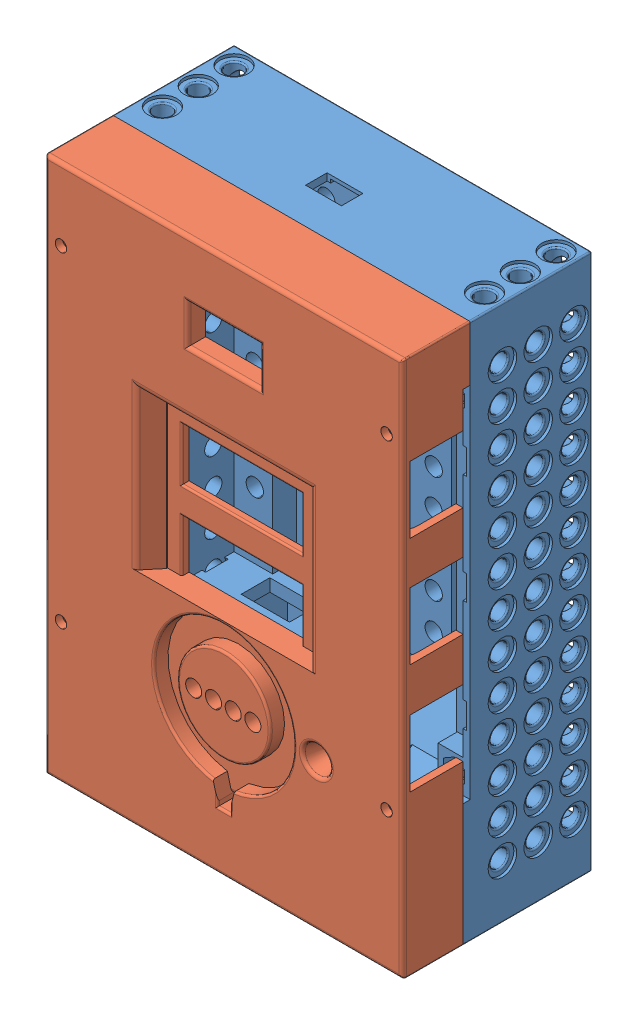
SolidWorks assembly _BRAIN_V3, configuration Default. Lengths in mm.
Overall size (100 150 52.91).
518 component instances, 29 part files, 8 mates.
Components (placement in the parent):
- RevvyDemoPCB-1: RevvyDemoPCB [Default] at (-47.0224 9.9913 94.3336) size (104.01 114.4 55.33) (hidden)
  - Board-1: Board [Default] at origin size (100 100 1.83)
  - C500-1: C500 [Default] at origin size (6.35 6.35 14.54)
    - SW3dPS-Cap_electro_6.3x11x2.5mm-1: SW3dPS-Cap_electro_6.3x11x2.5mm [Default] at (56.1999 84.3522 0) x (0 -1 0) z (-1 0 0) size (6.35 14.54 6.35)
  - R901-1: R901 [Default] at origin size (0.8 1.6 0.31)
    - 0603_SMD_Resistor-1: 0603_SMD_Resistor [Default] at (68.0999 7.3001 0) x (0 1 0) z (1 0 0) size (1.6 0.31 0.8)
  - U700-1: U700 [Default] at origin size (16.1 5.9 42.6)
    - User_Library-hc05-1: User_Library-hc05 [Default] at (15.5049 14.15 37) x (0 0 -1) z (0 -1 0) size (42.6 16.1 5.9) (hidden)
  - U500-1: U500 [Default] at origin size (6.5 7 1.7)
    - User_Library-SOT223-3-1: User_Library-SOT223-3 [Default] at (48.7999 82.0999 0) x (-1 0 0) z (0 0 1) size (6.5 7 1.7)
  - U405-1: U405 [Default] at origin size (10.01 6 1.76)
    - 1025808048-1: 1025808048 [Default] at (6 19.25 -1.8339) x (0 -1 0) z (0 0 -1) size (6 10.01 1.76)
      - Open_CASCADE_STEP_translator_6.8_1.1-1: Open_CASCADE_STEP_translator_6.8_1.1 [Default] at (-2 -5 0.001) size (0.5 0.5 0)
      - Body-1: Body [Default] at (-2 -5 0) size (4.01 10.01 1.51)
        - Open_CASCADE_STEP_translator_6.8_1.2.1-1: Open_CASCADE_STEP_translator_6.8_1.2.1 [Default] at origin size (4.01 10.01 1.51)
      - Leader-1: Leader [Default] at (-2 -4.445 0) x (-1 0 0) z (0 0 1) size (1 0.41 1.05)
      - Leader-2: Leader [Default] at (-2 -3.175 0) x (-1 0 0) z (0 0 1) size (1 0.41 1.05)
      - Leader-3: Leader [Default] at (-2 -1.905 0) x (-1 0 0) z (0 0 1) size (1 0.41 1.05)
      - Leader-4: Leader [Default] at (-2 -0.635 0) x (-1 0 0) z (0 0 1) size (1 0.41 1.05)
      - Leader-5: Leader [Default] at (-2 0.635 0) x (-1 0 0) z (0 0 1) size (1 0.41 1.05)
      - Leader-6: Leader [Default] at (-2 1.905 0) x (-1 0 0) z (0 0 1) size (1 0.41 1.05)
      - Leader-7: Leader [Default] at (-2 3.175 0) x (-1 0 0) z (0 0 1) size (1 0.41 1.05)
      - Leader-8: Leader [Default] at (-2 4.445 0) x (-1 0 0) z (0 0 1) size (1 0.41 1.05)
      - Leader-9: Leader [Default] at (2 -4.445 0) size (1 0.41 1.05)
      - Leader-10: Leader [Default] at (2 -3.175 0) size (1 0.41 1.05)
      - Leader-11: Leader [Default] at (2 -1.905 0) size (1 0.41 1.05)
      - Leader-12: Leader [Default] at (2 -0.635 0) size (1 0.41 1.05)
      - Leader-13: Leader [Default] at (2 0.635 0) size (1 0.41 1.05)
      - Leader-14: Leader [Default] at (2 1.905 0) size (1 0.41 1.05)
      - Leader-15: Leader [Default] at (2 3.175 0) size (1 0.41 1.05)
      - Leader-16: Leader [Default] at (2 4.445 0) size (1 0.41 1.05)
  - U404-1: U404 [Default] at origin size (10.01 6 1.76)
    - 1025808048-1: 1025808048 [Default] at (6 50.1 -1.8339) x (0 -1 0) z (0 0 -1) size (6 10.01 1.76)
      - Open_CASCADE_STEP_translator_6.8_1.1-1: Open_CASCADE_STEP_translator_6.8_1.1 [Default] at (-2 -5 0.001) size (0.5 0.5 0)
      - Body-1: Body [Default] at (-2 -5 0) size (4.01 10.01 1.51)
        - Open_CASCADE_STEP_translator_6.8_1.2.1-1: Open_CASCADE_STEP_translator_6.8_1.2.1 [Default] at origin size (4.01 10.01 1.51)
      - Leader-1: Leader [Default] at (-2 -4.445 0) x (-1 0 0) z (0 0 1) size (1 0.41 1.05)
      - Leader-2: Leader [Default] at (-2 -3.175 0) x (-1 0 0) z (0 0 1) size (1 0.41 1.05)
      - Leader-3: Leader [Default] at (-2 -1.905 0) x (-1 0 0) z (0 0 1) size (1 0.41 1.05)
      - Leader-4: Leader [Default] at (-2 -0.635 0) x (-1 0 0) z (0 0 1) size (1 0.41 1.05)
      - Leader-5: Leader [Default] at (-2 0.635 0) x (-1 0 0) z (0 0 1) size (1 0.41 1.05)
      - Leader-6: Leader [Default] at (-2 1.905 0) x (-1 0 0) z (0 0 1) size (1 0.41 1.05)
      - Leader-7: Leader [Default] at (-2 3.175 0) x (-1 0 0) z (0 0 1) size (1 0.41 1.05)
      - Leader-8: Leader [Default] at (-2 4.445 0) x (-1 0 0) z (0 0 1) size (1 0.41 1.05)
      - Leader-9: Leader [Default] at (2 -4.445 0) size (1 0.41 1.05)
      - Leader-10: Leader [Default] at (2 -3.175 0) size (1 0.41 1.05)
      - Leader-11: Leader [Default] at (2 -1.905 0) size (1 0.41 1.05)
      - Leader-12: Leader [Default] at (2 -0.635 0) size (1 0.41 1.05)
      - Leader-13: Leader [Default] at (2 0.635 0) size (1 0.41 1.05)
      - Leader-14: Leader [Default] at (2 1.905 0) size (1 0.41 1.05)
      - Leader-15: Leader [Default] at (2 3.175 0) size (1 0.41 1.05)
      - Leader-16: Leader [Default] at (2 4.445 0) size (1 0.41 1.05)
  - U403-1: U403 [Default] at origin size (10.01 6 1.76)
    - 1025808048-1: 1025808048 [Default] at (6 81 -1.8339) x (0 -1 0) z (0 0 -1) size (6 10.01 1.76)
      - Open_CASCADE_STEP_translator_6.8_1.1-1: Open_CASCADE_STEP_translator_6.8_1.1 [Default] at (-2 -5 0.001) size (0.5 0.5 0)
      - Body-1: Body [Default] at (-2 -5 0) size (4.01 10.01 1.51)
        - Open_CASCADE_STEP_translator_6.8_1.2.1-1: Open_CASCADE_STEP_translator_6.8_1.2.1 [Default] at origin size (4.01 10.01 1.51)
      - Leader-1: Leader [Default] at (-2 -4.445 0) x (-1 0 0) z (0 0 1) size (1 0.41 1.05)
      - Leader-2: Leader [Default] at (-2 -3.175 0) x (-1 0 0) z (0 0 1) size (1 0.41 1.05)
      - Leader-3: Leader [Default] at (-2 -1.905 0) x (-1 0 0) z (0 0 1) size (1 0.41 1.05)
      - Leader-4: Leader [Default] at (-2 -0.635 0) x (-1 0 0) z (0 0 1) size (1 0.41 1.05)
      - Leader-5: Leader [Default] at (-2 0.635 0) x (-1 0 0) z (0 0 1) size (1 0.41 1.05)
      - Leader-6: Leader [Default] at (-2 1.905 0) x (-1 0 0) z (0 0 1) size (1 0.41 1.05)
      - Leader-7: Leader [Default] at (-2 3.175 0) x (-1 0 0) z (0 0 1) size (1 0.41 1.05)
      - Leader-8: Leader [Default] at (-2 4.445 0) x (-1 0 0) z (0 0 1) size (1 0.41 1.05)
      - Leader-9: Leader [Default] at (2 -4.445 0) size (1 0.41 1.05)
      - Leader-10: Leader [Default] at (2 -3.175 0) size (1 0.41 1.05)
      - Leader-11: Leader [Default] at (2 -1.905 0) size (1 0.41 1.05)
      - Leader-12: Leader [Default] at (2 -0.635 0) size (1 0.41 1.05)
      - Leader-13: Leader [Default] at (2 0.635 0) size (1 0.41 1.05)
      - Leader-14: Leader [Default] at (2 1.905 0) size (1 0.41 1.05)
      - Leader-15: Leader [Default] at (2 3.175 0) size (1 0.41 1.05)
      - Leader-16: Leader [Default] at (2 4.445 0) size (1 0.41 1.05)
  - U402-1: U402 [Default] at origin size (10.01 6 1.76)
    - 1025808176-1: 1025808176 [Default] at (94 19.5 -1.8339) x (0 1 0) z (0 0 -1) size (6 10.01 1.76)
      - Open_CASCADE_STEP_translator_6.8_1.1_2-1: Open_CASCADE_STEP_translator_6.8_1.1_2 [Default] at (-2 -5 0.001) size (0.5 0.5 0)
      - Body_2-1: Body_2 [Default] at (-2 -5 0) size (4.01 10.01 1.51)
        - Open_CASCADE_STEP_translator_6.8_1.2.1_2-1: Open_CASCADE_STEP_translator_6.8_1.2.1_2 [Default] at origin size (4.01 10.01 1.51)
      - Leader_2-1: Leader_2 [Default] at (-2 -4.445 0) x (-1 0 0) z (0 0 1) size (1 0.41 1.05)
      - Leader_2-2: Leader_2 [Default] at (-2 -3.175 0) x (-1 0 0) z (0 0 1) size (1 0.41 1.05)
      - Leader_2-3: Leader_2 [Default] at (-2 -1.905 0) x (-1 0 0) z (0 0 1) size (1 0.41 1.05)
      - Leader_2-4: Leader_2 [Default] at (-2 -0.635 0) x (-1 0 0) z (0 0 1) size (1 0.41 1.05)
      - Leader_2-5: Leader_2 [Default] at (-2 0.635 0) x (-1 0 0) z (0 0 1) size (1 0.41 1.05)
      - Leader_2-6: Leader_2 [Default] at (-2 1.905 0) x (-1 0 0) z (0 0 1) size (1 0.41 1.05)
      - Leader_2-7: Leader_2 [Default] at (-2 3.175 0) x (-1 0 0) z (0 0 1) size (1 0.41 1.05)
      - Leader_2-8: Leader_2 [Default] at (-2 4.445 0) x (-1 0 0) z (0 0 1) size (1 0.41 1.05)
      - Leader_2-9: Leader_2 [Default] at (2 -4.445 0) size (1 0.41 1.05)
      - Leader_2-10: Leader_2 [Default] at (2 -3.175 0) size (1 0.41 1.05)
      - Leader_2-11: Leader_2 [Default] at (2 -1.905 0) size (1 0.41 1.05)
      - Leader_2-12: Leader_2 [Default] at (2 -0.635 0) size (1 0.41 1.05)
      - Leader_2-13: Leader_2 [Default] at (2 0.635 0) size (1 0.41 1.05)
      - Leader_2-14: Leader_2 [Default] at (2 1.905 0) size (1 0.41 1.05)
      - Leader_2-15: Leader_2 [Default] at (2 3.175 0) size (1 0.41 1.05)
      - Leader_2-16: Leader_2 [Default] at (2 4.445 0) size (1 0.41 1.05)
  - U401-1: U401 [Default] at origin size (10.01 6 1.76)
    - 1025808176-1: 1025808176 [Default] at (94 50.3 -1.8339) x (0 1 0) z (0 0 -1) size (6 10.01 1.76)
      - Open_CASCADE_STEP_translator_6.8_1.1_2-1: Open_CASCADE_STEP_translator_6.8_1.1_2 [Default] at (-2 -5 0.001) size (0.5 0.5 0)
      - Body_2-1: Body_2 [Default] at (-2 -5 0) size (4.01 10.01 1.51)
        - Open_CASCADE_STEP_translator_6.8_1.2.1_2-1: Open_CASCADE_STEP_translator_6.8_1.2.1_2 [Default] at origin size (4.01 10.01 1.51)
      - Leader_2-1: Leader_2 [Default] at (-2 -4.445 0) x (-1 0 0) z (0 0 1) size (1 0.41 1.05)
      - Leader_2-2: Leader_2 [Default] at (-2 -3.175 0) x (-1 0 0) z (0 0 1) size (1 0.41 1.05)
      - Leader_2-3: Leader_2 [Default] at (-2 -1.905 0) x (-1 0 0) z (0 0 1) size (1 0.41 1.05)
      - Leader_2-4: Leader_2 [Default] at (-2 -0.635 0) x (-1 0 0) z (0 0 1) size (1 0.41 1.05)
      - Leader_2-5: Leader_2 [Default] at (-2 0.635 0) x (-1 0 0) z (0 0 1) size (1 0.41 1.05)
      - Leader_2-6: Leader_2 [Default] at (-2 1.905 0) x (-1 0 0) z (0 0 1) size (1 0.41 1.05)
      - Leader_2-7: Leader_2 [Default] at (-2 3.175 0) x (-1 0 0) z (0 0 1) size (1 0.41 1.05)
      - Leader_2-8: Leader_2 [Default] at (-2 4.445 0) x (-1 0 0) z (0 0 1) size (1 0.41 1.05)
      - Leader_2-9: Leader_2 [Default] at (2 -4.445 0) size (1 0.41 1.05)
      - Leader_2-10: Leader_2 [Default] at (2 -3.175 0) size (1 0.41 1.05)
      - Leader_2-11: Leader_2 [Default] at (2 -1.905 0) size (1 0.41 1.05)
      - Leader_2-12: Leader_2 [Default] at (2 -0.635 0) size (1 0.41 1.05)
      - Leader_2-13: Leader_2 [Default] at (2 0.635 0) size (1 0.41 1.05)
      - Leader_2-14: Leader_2 [Default] at (2 1.905 0) size (1 0.41 1.05)
      - Leader_2-15: Leader_2 [Default] at (2 3.175 0) size (1 0.41 1.05)
      - Leader_2-16: Leader_2 [Default] at (2 4.445 0) size (1 0.41 1.05)
  - U400-1: U400 [Default] at origin size (10.01 6 1.76)
    - 1025808176-1: 1025808176 [Default] at (94 81.1 -1.8339) x (0 1 0) z (0 0 -1) size (6 10.01 1.76)
      - Open_CASCADE_STEP_translator_6.8_1.1_2-1: Open_CASCADE_STEP_translator_6.8_1.1_2 [Default] at (-2 -5 0.001) size (0.5 0.5 0)
      - Body_2-1: Body_2 [Default] at (-2 -5 0) size (4.01 10.01 1.51)
        - Open_CASCADE_STEP_translator_6.8_1.2.1_2-1: Open_CASCADE_STEP_translator_6.8_1.2.1_2 [Default] at origin size (4.01 10.01 1.51)
      - Leader_2-1: Leader_2 [Default] at (-2 -4.445 0) x (-1 0 0) z (0 0 1) size (1 0.41 1.05)
      - Leader_2-2: Leader_2 [Default] at (-2 -3.175 0) x (-1 0 0) z (0 0 1) size (1 0.41 1.05)
      - Leader_2-3: Leader_2 [Default] at (-2 -1.905 0) x (-1 0 0) z (0 0 1) size (1 0.41 1.05)
      - Leader_2-4: Leader_2 [Default] at (-2 -0.635 0) x (-1 0 0) z (0 0 1) size (1 0.41 1.05)
      - Leader_2-5: Leader_2 [Default] at (-2 0.635 0) x (-1 0 0) z (0 0 1) size (1 0.41 1.05)
      - Leader_2-6: Leader_2 [Default] at (-2 1.905 0) x (-1 0 0) z (0 0 1) size (1 0.41 1.05)
      - Leader_2-7: Leader_2 [Default] at (-2 3.175 0) x (-1 0 0) z (0 0 1) size (1 0.41 1.05)
      - Leader_2-8: Leader_2 [Default] at (-2 4.445 0) x (-1 0 0) z (0 0 1) size (1 0.41 1.05)
      - Leader_2-9: Leader_2 [Default] at (2 -4.445 0) size (1 0.41 1.05)
      - Leader_2-10: Leader_2 [Default] at (2 -3.175 0) size (1 0.41 1.05)
      - Leader_2-11: Leader_2 [Default] at (2 -1.905 0) size (1 0.41 1.05)
      - Leader_2-12: Leader_2 [Default] at (2 -0.635 0) size (1 0.41 1.05)
      - Leader_2-13: Leader_2 [Default] at (2 0.635 0) size (1 0.41 1.05)
      - Leader_2-14: Leader_2 [Default] at (2 1.905 0) size (1 0.41 1.05)
      - Leader_2-15: Leader_2 [Default] at (2 3.175 0) size (1 0.41 1.05)
      - Leader_2-16: Leader_2 [Default] at (2 4.445 0) size (1 0.41 1.05)
  - SW500-1: SW500 [Default] at origin size (17.2 10.8 12.4)
    - 859988520-1: 859988520 [Default] at (48.5 94.1 0) size (17.2 10.8 12.4)
      - Extruded-1: Extruded [Default] at origin size (17.2 10.8 12.4)
  - R900-1: R900 [Default] at origin size (0.8 1.6 0.31)
    - 0603_SMD_Resistor-1: 0603_SMD_Resistor [Default] at (86.8001 6.7001 -1.8339) x (0 1 0) z (-1 0 0) size (1.6 0.31 0.8)
  - R841-1: R841 [Default] at origin size (1.6 0.8 0.31)
    - 0603_SMD_Resistor-1: 0603_SMD_Resistor [Default] at (64.7501 62.0499 -1.8339) x (1 0 0) z (0 1 0) size (1.6 0.31 0.8)
  - R840-1: R840 [Default] at origin size (0.8 1.6 0.31)
    - 0603_SMD_Resistor-1: 0603_SMD_Resistor [Default] at (76.9501 86.1999 0) x (0 -1 0) z (-1 0 0) size (1.6 0.31 0.8)
  - R839-1: R839 [Default] at origin size (1.6 0.8 0.31)
    - 0603_SMD_Resistor-1: 0603_SMD_Resistor [Default] at (56.7999 60.1001 -1.8339) x (-1 0 0) z (0 -1 0) size (1.6 0.31 0.8)
  - R838-1: R838 [Default] at origin size (1.6 0.8 0.31)
    - 0603_SMD_Resistor-1: 0603_SMD_Resistor [Default] at (56.7999 62.1001 -1.8339) x (-1 0 0) z (0 -1 0) size (1.6 0.31 0.8)
  - R837-1: R837 [Default] at origin size (0.8 1.6 0.31)
    - 0603_SMD_Resistor-1: 0603_SMD_Resistor [Default] at (81.9999 64.0501 0) x (0 1 0) z (1 0 0) size (1.6 0.31 0.8)
  - R836-1: R836 [Default] at origin size (1.6 0.8 0.31)
    - 0603_SMD_Resistor-1: 0603_SMD_Resistor [Default] at (56.7001 49.2999 -1.8339) x (1 0 0) z (0 1 0) size (1.6 0.31 0.8)
  - R835-1: R835 [Default] at origin size (1.6 0.8 0.31)
    - 0603_SMD_Resistor-1: 0603_SMD_Resistor [Default] at (64.7999 68.7001 -1.8339) x (-1 0 0) z (0 -1 0) size (1.6 0.31 0.8)
  - R834-1: R834 [Default] at origin size (1.6 0.8 0.31)
    - 0603_SMD_Resistor-1: 0603_SMD_Resistor [Default] at (64.6001 53.0999 -1.8339) x (1 0 0) z (0 1 0) size (1.6 0.31 0.8)
  - R833-1: R833 [Default] at origin size (1.6 0.8 0.31)
    - 0603_SMD_Resistor-1: 0603_SMD_Resistor [Default] at (63.5001 70.4999 -1.8339) x (1 0 0) z (0 1 0) size (1.6 0.31 0.8)
  - R832-1: R832 [Default] at origin size (1.6 0.8 0.31)
    - 0603_SMD_Resistor-1: 0603_SMD_Resistor [Default] at (65.6001 24.1999 -1.8339) x (1 0 0) z (0 1 0) size (1.6 0.31 0.8)
  - R831-1: R831 [Default] at origin size (1.6 0.8 0.31)
    - 0603_SMD_Resistor-1: 0603_SMD_Resistor [Default] at (65.6001 31.7999 -1.8339) x (1 0 0) z (0 1 0) size (1.6 0.31 0.8)
  - R830-1: R830 [Default] at origin size (1.6 0.8 0.31)
    - 0603_SMD_Resistor-1: 0603_SMD_Resistor [Default] at (65.5001 27.8999 -1.8339) x (1 0 0) z (0 1 0) size (1.6 0.31 0.8)
  - R829-1: R829 [Default] at origin size (1.6 0.8 0.31)
    - 0603_SMD_Resistor-1: 0603_SMD_Resistor [Default] at (56.7999 68.7001 -1.8339) x (-1 0 0) z (0 -1 0) size (1.6 0.31 0.8)
  - R828-1: R828 [Default] at origin size (1.6 0.8 0.31)
    - 0603_SMD_Resistor-1: 0603_SMD_Resistor [Default] at (41.7999 43.4001 -1.8339) x (-1 0 0) z (0 -1 0) size (1.6 0.31 0.8)
  - R827-1: R827 [Default] at origin size (1.6 0.8 0.31)
    - 0603_SMD_Resistor-1: 0603_SMD_Resistor [Default] at (20.1001 37.2999 -1.8339) x (1 0 0) z (0 1 0) size (1.6 0.31 0.8)
  - R826-1: R826 [Default] at origin size (1.6 0.8 0.31)
    - 0603_SMD_Resistor-1: 0603_SMD_Resistor [Default] at (56.7999 70.7001 -1.8339) x (-1 0 0) z (0 -1 0) size (1.6 0.31 0.8)
  - R825-1: R825 [Default] at origin size (1.6 0.8 0.31)
    - 0603_SMD_Resistor-1: 0603_SMD_Resistor [Default] at (56.7001 52.9999 -1.8339) x (1 0 0) z (0 1 0) size (1.6 0.31 0.8)
  - R824-1: R824 [Default] at origin size (1.6 0.8 0.31)
    - 0603_SMD_Resistor-1: 0603_SMD_Resistor [Default] at (56.8001 65.8999 -1.8339) x (1 0 0) z (0 1 0) size (1.6 0.31 0.8)
  - R823-1: R823 [Default] at origin size (1.6 0.8 0.31)
    - 0603_SMD_Resistor-1: 0603_SMD_Resistor [Default] at (33.8502 51.8001 -1.8339) x (-1 0 0) z (0 -1 0) size (1.6 0.31 0.8)
  - R822-1: R822 [Default] at origin size (1.6 0.8 0.31)
    - 0603_SMD_Resistor-1: 0603_SMD_Resistor [Default] at (64.7999 73.2001 -1.8339) x (-1 0 0) z (0 -1 0) size (1.6 0.31 0.8)
  - R821-1: R821 [Default] at origin size (1.6 0.8 0.31)
    - 0603_SMD_Resistor-1: 0603_SMD_Resistor [Default] at (64.7999 75.2001 -1.8339) x (-1 0 0) z (0 -1 0) size (1.6 0.31 0.8)
  - R820-1: R820 [Default] at origin size (1.6 0.8 0.31)
    - 0603_SMD_Resistor-1: 0603_SMD_Resistor [Default] at (57.5001 29.8999 -1.8339) x (1 0 0) z (0 1 0) size (1.6 0.31 0.8)
  - R819-1: R819 [Default] at origin size (1.6 0.8 0.31)
    - 0603_SMD_Resistor-1: 0603_SMD_Resistor [Default] at (56.7001 45.3999 -1.8339) x (1 0 0) z (0 1 0) size (1.6 0.31 0.8)
  - R818-1: R818 [Default] at origin size (1.6 0.8 0.31)
    - 0603_SMD_Resistor-1: 0603_SMD_Resistor [Default] at (57.6001 33.8999 -1.8339) x (1 0 0) z (0 1 0) size (1.6 0.31 0.8)
  - R817-1: R817 [Default] at origin size (1.6 0.8 0.31)
    - 0603_SMD_Resistor-1: 0603_SMD_Resistor [Default] at (70.9001 59.8001 0) x (1 0 0) z (0 -1 0) size (1.6 0.31 0.8)
  - R816-1: R816 [Default] at origin size (1.6 0.8 0.31)
    - 0603_SMD_Resistor-1: 0603_SMD_Resistor [Default] at (56.7999 73.1001 -1.8339) x (-1 0 0) z (0 -1 0) size (1.6 0.31 0.8)
  - R815-1: R815 [Default] at origin size (1.6 0.8 0.31)
    - 0603_SMD_Resistor-1: 0603_SMD_Resistor [Default] at (41.6999 39.2001 -1.8339) x (-1 0 0) z (0 -1 0) size (1.6 0.31 0.8)
  - R814-1: R814 [Default] at origin size (1.6 0.8 0.31)
    - 0603_SMD_Resistor-1: 0603_SMD_Resistor [Default] at (20.1001 39.2999 -1.8339) x (1 0 0) z (0 1 0) size (1.6 0.31 0.8)
  - R813-1: R813 [Default] at origin size (1.6 0.8 0.31)
    - 0603_SMD_Resistor-1: 0603_SMD_Resistor [Default] at (56.7999 75.1001 -1.8339) x (-1 0 0) z (0 -1 0) size (1.6 0.31 0.8)
  - R812-1: R812 [Default] at origin size (1.6 0.8 0.31)
    - 0603_SMD_Resistor-1: 0603_SMD_Resistor [Default] at (33.8999 47.6001 -1.8339) x (-1 0 0) z (0 -1 0) size (1.6 0.31 0.8)
  - R811-1: R811 [Default] at origin size (1.6 0.8 0.31)
    - 0603_SMD_Resistor-1: 0603_SMD_Resistor [Default] at (79.1999 55.5999 0) x (-1 0 0) z (0 1 0) size (1.6 0.31 0.8)
  - R810-1: R810 [Default] at origin size (1.6 0.8 0.31)
    - 0603_SMD_Resistor-1: 0603_SMD_Resistor [Default] at (41.7999 51.8001 -1.8339) x (-1 0 0) z (0 -1 0) size (1.6 0.31 0.8)
  - R809-1: R809 [Default] at origin size (1.6 0.8 0.31)
    - 0603_SMD_Resistor-1: 0603_SMD_Resistor [Default] at (33.9001 26.4999 -1.8339) x (1 0 0) z (0 1 0) size (1.6 0.31 0.8)
  - R808-1: R808 [Default] at origin size (1.6 0.8 0.31)
    - 0603_SMD_Resistor-1: 0603_SMD_Resistor [Default] at (33.8999 24.6001 -1.8339) x (-1 0 0) z (0 -1 0) size (1.6 0.31 0.8)
  - R807-1: R807 [Default] at origin size (1.6 0.8 0.31)
    - 0603_SMD_Resistor-1: 0603_SMD_Resistor [Default] at (56.7001 56.9999 -1.8339) x (1 0 0) z (0 1 0) size (1.6 0.31 0.8)
  - R806-1: R806 [Default] at origin size (1.6 0.8 0.31)
    - 0603_SMD_Resistor-1: 0603_SMD_Resistor [Default] at (79.1999 50.4999 0) x (-1 0 0) z (0 1 0) size (1.6 0.31 0.8)
  - R805-1: R805 [Default] at origin size (1.6 0.8 0.31)
    - 0603_SMD_Resistor-1: 0603_SMD_Resistor [Default] at (65.6001 35.7999 -1.8339) x (1 0 0) z (0 1 0) size (1.6 0.31 0.8)
  - R804-1: R804 [Default] at origin size (1.6 0.8 0.31)
    - 0603_SMD_Resistor-1: 0603_SMD_Resistor [Default] at (33.8999 43.4001 -1.8339) x (-1 0 0) z (0 -1 0) size (1.6 0.31 0.8)
  - R803-1: R803 [Default] at origin size (1.6 0.8 0.31)
    - 0603_SMD_Resistor-1: 0603_SMD_Resistor [Default] at (33.9001 22.0999 -1.8339) x (1 0 0) z (0 1 0) size (1.6 0.31 0.8)
  - R802-1: R802 [Default] at origin size (1.6 0.8 0.31)
    - 0603_SMD_Resistor-1: 0603_SMD_Resistor [Default] at (20.1001 41.2999 -1.8339) x (1 0 0) z (0 1 0) size (1.6 0.31 0.8)
  - R801-1: R801 [Default] at origin size (1.6 0.8 0.31)
    - 0603_SMD_Resistor-1: 0603_SMD_Resistor [Default] at (33.9999 30.8001 -1.8339) x (-1 0 0) z (0 -1 0) size (1.6 0.31 0.8)
  - R800-1: R800 [Default] at origin size (1.6 0.8 0.31)
    - 0603_SMD_Resistor-1: 0603_SMD_Resistor [Default] at (33.8999 20.2001 -1.8339) x (-1 0 0) z (0 -1 0) size (1.6 0.31 0.8)
  - R600-1: R600 [Default] at origin size (1.6 0.8 0.31)
    - 0603_SMD_Resistor-1: 0603_SMD_Resistor [Default] at (36.8001 9.5001 0) x (1 0 0) z (0 -1 0) size (1.6 0.31 0.8)
  - R500-1: R500 [Default] at origin size (1.6 0.8 0.31)
    - 0603_SMD_Resistor-1: 0603_SMD_Resistor [Default] at (64.4999 91.7001 -1.8339) x (-1 0 0) z (0 -1 0) size (1.6 0.31 0.8)
  - Q900-1: Q900 [Default] at origin size (2.5 3 1.1)
    - CircuitWorks-SOT-23-1: CircuitWorks-SOT-23 [Default] at (83.1499 6.6499 -2.3839) x (0 1 0) z (-1 0 0) size (3 1.1 2.5)
  - Q500-1: Q500 [Default] at origin size (5 7.8 1.8)
    - User_Library-SOIC-8-1: User_Library-SOIC-8 [Default] at (60.4999 94.7001 0) x (1 0 0) z (0 -1 0) size (5 1.75 6.01)
      - User_Library-SOIC-8_SOIC-8_Body_1-1: User_Library-SOIC-8_SOIC-8_Body_1 [Default] at origin size (5 1.6 4)
      - User_Library-SOIC-8_SOIC-8_Pins_1-1: User_Library-SOIC-8_SOIC-8_Pins_1 [Default] at origin size (4.23 0.99 6.01)
    - 859988384-1: 859988384 [Default] at (60.5 94.7 0) size (5 7.8 1.8)
      - Extruded_2-1: Extruded_2 [Default] at origin size (5 7.8 1.8)
  - LED603-1: LED603 [Default] at origin size (5 5.4 1.7)
    - User_Library-WS2812B-1: User_Library-WS2812B [Default] at (58.1501 6.9999 0.2032) x (0 1 0) z (1 0 0) size (5.4 1.7 5)
  - LED602-1: LED602 [Default] at origin size (5 5.4 1.7)
    - User_Library-WS2812B-1: User_Library-WS2812B [Default] at (52.6334 6.9999 0.2032) x (0 1 0) z (1 0 0) size (5.4 1.7 5)
  - LED601-1: LED601 [Default] at origin size (5 5.4 1.7)
    - User_Library-WS2812B-1: User_Library-WS2812B [Default] at (47.1167 6.9999 0.2032) x (0 1 0) z (1 0 0) size (5.4 1.7 5)
  - LED600-1: LED600 [Default] at origin size (5 5.4 1.7)
    - User_Library-WS2812B-1: User_Library-WS2812B [Default] at (41.6001 6.9999 0.2032) x (0 1 0) z (1 0 0) size (5.4 1.7 5)
  - J300-1: J300 [Default] at origin size (65.5 102.57 23)
    - stm30f4-1: stm30f4 [Default] at (16.9359 15.8089 -4.8339) x (0 1 0) z (-1 0 0) size (102.57 23 65.5)
  - J209-1: J209 [Default] at origin size (15.76 18 12.81)
    - c-1-338088-3-z-3d-1: c-1-338088-3-z-3d [Default] at (58.2001 34.575 12.7) x (1 0 0) z (0 0 1) size (15.76 18 12.81)
  - J208-1: J208 [Default] at origin size (15.76 18 12.81)
    - c-1-338088-3-z-3d-1: c-1-338088-3-z-3d [Default] at (41.2001 34.575 12.7) x (1 0 0) z (0 0 1) size (15.76 18 12.81)
  - J207-1: J207 [Default] at origin size (15.76 18 12.81)
    - c-1-338088-3-z-3d-1: c-1-338088-3-z-3d [Default] at (58.1999 56.825 12.7) x (-1 0 0) z (0 0 1) size (15.76 18 12.81)
  - J206-1: J206 [Default] at origin size (15.76 18 12.81)
    - c-1-338088-3-z-3d-1: c-1-338088-3-z-3d [Default] at (41.1999 56.825 12.7) x (-1 0 0) z (0 0 1) size (15.76 18 12.81)
  - J205-1: J205 [Default] at origin size (16.48 18.8 15.93)
    - c-6339160-1-e-3d-1: c-6339160-1-e-3d [Default] at (102.0301 19.35 6.8) x (0 1 0) z (1 0 0) size (18.8 15.93 16.48)
  - J204-1: J204 [Default] at origin size (16.48 18.8 15.93)
    - c-6339160-1-e-3d-1: c-6339160-1-e-3d [Default] at (-1.9801 19.35 6.8) x (0 -1 0) z (-1 0 0) size (18.8 15.93 16.48)
  - J203-1: J203 [Default] at origin size (16.48 18.8 15.93)
    - c-6339160-1-e-3d-1: c-6339160-1-e-3d [Default] at (102.0301 50.147 6.8) x (0 1 0) z (1 0 0) size (18.8 15.93 16.48)
  - J202-1: J202 [Default] at origin size (16.48 18.8 15.93)
    - c-6339160-1-e-3d-1: c-6339160-1-e-3d [Default] at (-1.9801 50.1471 6.8) x (0 -1 0) z (-1 0 0) size (18.8 15.93 16.48)
  - J201-1: J201 [Default] at origin size (16.48 18.8 15.93)
    - c-6339160-1-e-3d-1: c-6339160-1-e-3d [Default] at (102.0301 80.75 6.8) x (0 1 0) z (1 0 0) size (18.8 15.93 16.48)
  - J200-1: J200 [Default] at origin size (16.48 18.8 15.93)
    - c-6339160-1-e-3d-1: c-6339160-1-e-3d [Default] at (-1.9801 80.75 6.8) x (0 -1 0) z (-1 0 0) size (18.8 15.93 16.48)
  - D833-1: D833 [Default] at origin size (2.5 3 1.1)
    - CircuitWorks-SOT-23-1: CircuitWorks-SOT-23 [Default] at (68.2001 61.1001 -2.3839) x (0 -1 0) z (1 0 0) size (3 1.1 2.5)
  - D832-1: D832 [Default] at origin size (2.5 3 1.1)
    - CircuitWorks-SOT-23-1: CircuitWorks-SOT-23 [Default] at (60.2501 61.1001 -2.3839) x (0 -1 0) z (1 0 0) size (3 1.1 2.5)
  - D831-1: D831 [Default] at origin size (2.5 3 1.1)
    - CircuitWorks-SOT-23-1: CircuitWorks-SOT-23 [Default] at (68.2501 65.9001 -2.3839) x (0 -1 0) z (1 0 0) size (3 1.1 2.5)
  - D830-1: D830 [Default] at origin size (2.5 3 1.1)
    - CircuitWorks-SOT-23-1: CircuitWorks-SOT-23 [Default] at (60.1501 49.3001 -2.3839) x (0 -1 0) z (1 0 0) size (3 1.1 2.5)
  - D829-1: D829 [Default] at origin size (2.5 3 1.1)
    - CircuitWorks-SOT-23-1: CircuitWorks-SOT-23 [Default] at (68.2501 69.7001 -2.3839) x (0 -1 0) z (1 0 0) size (3 1.1 2.5)
  - D828-1: D828 [Default] at origin size (2.5 3 1.1)
    - CircuitWorks-SOT-23-1: CircuitWorks-SOT-23 [Default] at (69.0501 24.2001 -2.3839) x (0 -1 0) z (1 0 0) size (3 1.1 2.5)
  - D827-1: D827 [Default] at origin size (2.5 3 1.1)
    - CircuitWorks-SOT-23-1: CircuitWorks-SOT-23 [Default] at (69.0501 31.8001 -2.3839) x (0 -1 0) z (1 0 0) size (3 1.1 2.5)
  - D826-1: D826 [Default] at origin size (2.5 3 1.1)
    - CircuitWorks-SOT-23-1: CircuitWorks-SOT-23 [Default] at (68.1501 53.1001 -2.3839) x (0 -1 0) z (1 0 0) size (3 1.1 2.5)
  - D825-1: D825 [Default] at origin size (2.5 3 1.1)
    - CircuitWorks-SOT-23-1: CircuitWorks-SOT-23 [Default] at (38.3499 43.3999 -2.3839) x (0 1 0) z (-1 0 0) size (3 1.1 2.5)
  - D824-1: D824 [Default] at origin size (2.5 3 1.1)
    - CircuitWorks-SOT-23-1: CircuitWorks-SOT-23 [Default] at (38.2499 34.9999 -2.3839) x (0 1 0) z (-1 0 0) size (3 1.1 2.5)
  - D823-1: D823 [Default] at origin size (2.5 3 1.1)
    - CircuitWorks-SOT-23-1: CircuitWorks-SOT-23 [Default] at (69.0501 27.9001 -2.3839) x (0 -1 0) z (1 0 0) size (3 1.1 2.5)
  - D822-1: D822 [Default] at origin size (2.5 3 1.1)
    - CircuitWorks-SOT-23-1: CircuitWorks-SOT-23 [Default] at (60.2501 69.7001 -2.3839) x (0 -1 0) z (1 0 0) size (3 1.1 2.5)
  - D821-1: D821 [Default] at origin size (2.5 3 1.1)
    - CircuitWorks-SOT-23-1: CircuitWorks-SOT-23 [Default] at (60.2501 65.9001 -2.3839) x (0 -1 0) z (1 0 0) size (3 1.1 2.5)
  - D820-1: D820 [Default] at origin size (2.5 3 1.1)
    - CircuitWorks-SOT-23-1: CircuitWorks-SOT-23 [Default] at (30.4001 51.7999 -2.3839) x (0 1 0) z (-1 0 0) size (3 1.1 2.5)
  - D819-1: D819 [Default] at origin size (2.5 3 1.1)
    - CircuitWorks-SOT-23-1: CircuitWorks-SOT-23 [Default] at (60.1501 53.0001 -2.3839) x (0 -1 0) z (1 0 0) size (3 1.1 2.5)
  - D818-1: D818 [Default] at origin size (2.5 3 1.1)
    - CircuitWorks-SOT-23-1: CircuitWorks-SOT-23 [Default] at (68.2501 74.2001 -2.3839) x (0 -1 0) z (1 0 0) size (3 1.1 2.5)
  - D817-1: D817 [Default] at origin size (2.5 3 1.1)
    - CircuitWorks-SOT-23-1: CircuitWorks-SOT-23 [Default] at (60.1501 45.4001 -2.3839) x (0 -1 0) z (1 0 0) size (3 1.1 2.5)
  - D816-1: D816 [Default] at origin size (2.5 3 1.1)
    - CircuitWorks-SOT-23-1: CircuitWorks-SOT-23 [Default] at (61.0501 33.9001 -2.3839) x (0 -1 0) z (1 0 0) size (3 1.1 2.5)
  - D815-1: D815 [Default] at origin size (2.5 3 1.1)
    - CircuitWorks-SOT-23-1: CircuitWorks-SOT-23 [Default] at (61.0501 29.9001 -2.3839) x (0 -1 0) z (1 0 0) size (3 1.1 2.5)
  - D814-1: D814 [Default] at origin size (2.5 3 1.1)
    - CircuitWorks-SOT-23-1: CircuitWorks-SOT-23 [Default] at (38.2499 39.1999 -2.3839) x (0 1 0) z (-1 0 0) size (3 1.1 2.5)
  - D813-1: D813 [Default] at origin size (2.5 3 1.1)
    - CircuitWorks-SOT-23-1: CircuitWorks-SOT-23 [Default] at (30.4826 35.0159 -2.3839) x (0 1 0) z (-1 0 0) size (3 1.1 2.5)
  - D812-1: D812 [Default] at origin size (2.5 3 1.1)
    - CircuitWorks-SOT-23-1: CircuitWorks-SOT-23 [Default] at (68.1501 57.1001 -2.3839) x (0 -1 0) z (1 0 0) size (3 1.1 2.5)
  - D811-1: D811 [Default] at origin size (2.5 3 1.1)
    - CircuitWorks-SOT-23-1: CircuitWorks-SOT-23 [Default] at (60.2999 74.0988 -2.3839) x (0 -1 0) z (1 0 0) size (3 1.1 2.5)
  - D810-1: D810 [Default] at origin size (2.5 3 1.1)
    - CircuitWorks-SOT-23-1: CircuitWorks-SOT-23 [Default] at (68.1501 49.3001 -2.3839) x (0 -1 0) z (1 0 0) size (3 1.1 2.5)
  - D809-1: D809 [Default] at origin size (2.5 3 1.1)
    - CircuitWorks-SOT-23-1: CircuitWorks-SOT-23 [Default] at (38.3499 51.7999 -2.3839) x (0 1 0) z (-1 0 0) size (3 1.1 2.5)
  - D808-1: D808 [Default] at origin size (2.5 3 1.1)
    - CircuitWorks-SOT-23-1: CircuitWorks-SOT-23 [Default] at (30.4499 47.5999 -2.3839) x (0 1 0) z (-1 0 0) size (3 1.1 2.5)
  - D807-1: D807 [Default] at origin size (2.5 3 1.1)
    - CircuitWorks-SOT-23-1: CircuitWorks-SOT-23 [Default] at (30.4499 25.4999 -2.3839) x (0 1 0) z (-1 0 0) size (3 1.1 2.5)
  - D806-1: D806 [Default] at origin size (2.5 3 1.1)
    - CircuitWorks-SOT-23-1: CircuitWorks-SOT-23 [Default] at (68.1501 45.4001 -2.3839) x (0 -1 0) z (1 0 0) size (3 1.1 2.5)
  - D805-1: D805 [Default] at origin size (2.5 3 1.1)
    - CircuitWorks-SOT-23-1: CircuitWorks-SOT-23 [Default] at (69.0501 35.8001 -2.3839) x (0 -1 0) z (1 0 0) size (3 1.1 2.5)
  - D804-1: D804 [Default] at origin size (2.5 3 1.1)
    - CircuitWorks-SOT-23-1: CircuitWorks-SOT-23 [Default] at (60.1501 57.1001 -2.3839) x (0 -1 0) z (1 0 0) size (3 1.1 2.5)
  - D803-1: D803 [Default] at origin size (2.5 3 1.1)
    - CircuitWorks-SOT-23-1: CircuitWorks-SOT-23 [Default] at (30.4499 39.1999 -2.3839) x (0 1 0) z (-1 0 0) size (3 1.1 2.5)
  - D802-1: D802 [Default] at origin size (2.5 3 1.1)
    - CircuitWorks-SOT-23-1: CircuitWorks-SOT-23 [Default] at (30.4499 30.7999 -2.3839) x (0 1 0) z (-1 0 0) size (3 1.1 2.5)
  - D801-1: D801 [Default] at origin size (2.5 3 1.1)
    - CircuitWorks-SOT-23-1: CircuitWorks-SOT-23 [Default] at (30.4499 43.3999 -2.3839) x (0 1 0) z (-1 0 0) size (3 1.1 2.5)
  - D800-1: D800 [Default] at origin size (2.5 3 1.1)
    - CircuitWorks-SOT-23-1: CircuitWorks-SOT-23 [Default] at (30.4499 21.1999 -2.3839) x (0 1 0) z (-1 0 0) size (3 1.1 2.5)
  - D501-1: D501 [Default] at origin size (5.3 3.7 2.25)
    - User_Library-DO-214AA_SMB-1: User_Library-DO-214AA_SMB [Default] at (61.1001 88.0999 -1.8839) x (-1 0 0) z (0 0 -1) size (5.3 3.7 2.25)
  - D500-1: D500 [Default] at origin size (3.85 1.71 1.45)
    - User_Library-SOD-123_DiodesInc-1: User_Library-SOD-123_DiodesInc [Default] at (59.2749 96.1501 -2.3539) x (1 0 0) z (0 0 -1) size (3.85 1.71 1.45)
  - C823-1: C823 [Default] at origin size (2.3 1.1 0.9)
    - User_Library-CAPC1608X09-1: User_Library-CAPC1608X09 [Default] at (79.2001 63.6 0) x (1 0 0) z (0 0 1) size (1.6 0.8 0.9)
    - 859988112-1: 859988112 [Default] at (79.2 63.6 0) size (2.3 1.1 0.9)
      - Extruded_3-1: Extruded_3 [Default] at origin size (2.3 1.1 0.9)
  - C822-1: C822 [Default] at origin size (2.3 1.1 0.9)
    - User_Library-CAPC1608X09-1: User_Library-CAPC1608X09 [Default] at (70.8999 63.6 0) x (-1 0 0) z (0 0 1) size (1.6 0.8 0.9)
    - 859988112-1: 859988112 [Default] at (70.9 63.6 0) size (2.3 1.1 0.9)
      - Extruded_3-1: Extruded_3 [Default] at origin size (2.3 1.1 0.9)
  - C821-1: C821 [Default] at origin size (2.3 1.1 0.9)
    - User_Library-CAPC1608X09-1: User_Library-CAPC1608X09 [Default] at (79.2001 66.2 0) x (1 0 0) z (0 0 1) size (1.6 0.8 0.9)
    - 859988112-1: 859988112 [Default] at (79.2 66.2 0) size (2.3 1.1 0.9)
      - Extruded_3-1: Extruded_3 [Default] at origin size (2.3 1.1 0.9)
  - C820-1: C820 [Default] at origin size (2.3 1.1 0.9)
    - User_Library-CAPC1608X09-1: User_Library-CAPC1608X09 [Default] at (70.8999 53.4 0) x (-1 0 0) z (0 0 1) size (1.6 0.8 0.9)
    - 859988112-1: 859988112 [Default] at (70.9 53.4 0) size (2.3 1.1 0.9)
      - Extruded_3-1: Extruded_3 [Default] at origin size (2.3 1.1 0.9)
  - C819-1: C819 [Default] at origin size (2.3 1.1 0.9)
    - User_Library-CAPC1608X09-1: User_Library-CAPC1608X09 [Default] at (79.2001 68.7 0) x (1 0 0) z (0 0 1) size (1.6 0.8 0.9)
    - 859988112-1: 859988112 [Default] at (79.2 68.7 0) size (2.3 1.1 0.9)
      - Extruded_3-1: Extruded_3 [Default] at origin size (2.3 1.1 0.9)
  - C818-1: C818 [Default] at origin size (2.3 1.1 0.9)
    - User_Library-CAPC1608X09-1: User_Library-CAPC1608X09 [Default] at (70.8999 28.1 0) x (-1 0 0) z (0 0 1) size (1.6 0.8 0.9)
    - 859988112-1: 859988112 [Default] at (70.9 28.1 0) size (2.3 1.1 0.9)
      - Extruded_3-1: Extruded_3 [Default] at origin size (2.3 1.1 0.9)
  - C817-1: C817 [Default] at origin size (2.3 1.1 0.9)
    - User_Library-CAPC1608X09-1: User_Library-CAPC1608X09 [Default] at (70.8999 33.1 0) x (-1 0 0) z (0 0 1) size (1.6 0.8 0.9)
    - 859988112-1: 859988112 [Default] at (70.9 33.1 0) size (2.3 1.1 0.9)
      - Extruded_3-1: Extruded_3 [Default] at origin size (2.3 1.1 0.9)
  - C816-1: C816 [Default] at origin size (2.3 1.1 0.9)
    - User_Library-CAPC1608X09-1: User_Library-CAPC1608X09 [Default] at (28.4001 43.3 0) x (1 0 0) z (0 0 1) size (1.6 0.8 0.9)
    - 859988112-1: 859988112 [Default] at (28.4 43.3 0) size (2.3 1.1 0.9)
      - Extruded_3-1: Extruded_3 [Default] at origin size (2.3 1.1 0.9)
  - C815-1: C815 [Default] at origin size (2.3 1.1 0.9)
    - User_Library-CAPC1608X09-1: User_Library-CAPC1608X09 [Default] at (20.0999 38.2 0) x (-1 0 0) z (0 0 1) size (1.6 0.8 0.9)
    - 859988112-1: 859988112 [Default] at (20.1 38.2 0) size (2.3 1.1 0.9)
      - Extruded_3-1: Extruded_3 [Default] at origin size (2.3 1.1 0.9)
  - C814-1: C814 [Default] at origin size (2.3 1.1 0.9)
    - User_Library-CAPC1608X09-1: User_Library-CAPC1608X09 [Default] at (70.8999 68.7 0) x (-1 0 0) z (0 0 1) size (1.6 0.8 0.9)
    - 859988112-1: 859988112 [Default] at (70.9 68.7 0) size (2.3 1.1 0.9)
      - Extruded_3-1: Extruded_3 [Default] at origin size (2.3 1.1 0.9)
  - C813-1: C813 [Default] at origin size (2.3 1.1 0.9)
    - User_Library-CAPC1608X09-1: User_Library-CAPC1608X09 [Default] at (70.8999 66.2 0) x (-1 0 0) z (0 0 1) size (1.6 0.8 0.9)
    - 859988112-1: 859988112 [Default] at (70.9 66.2 0) size (2.3 1.1 0.9)
      - Extruded_3-1: Extruded_3 [Default] at origin size (2.3 1.1 0.9)
  - C812-1: C812 [Default] at origin size (2.3 1.1 0.9)
    - User_Library-CAPC1608X09-1: User_Library-CAPC1608X09 [Default] at (20.0999 48.4 -1.8339) x (-1 0 0) z (0 0 -1) size (1.6 0.8 0.9)
    - 859988112-1: 859988112 [Default] at (20.1 48.4 -2.7339) size (2.3 1.1 0.9)
      - Extruded_3-1: Extruded_3 [Default] at origin size (2.3 1.1 0.9)
  - C811-1: C811 [Default] at origin size (2.3 1.1 0.9)
    - User_Library-CAPC1608X09-1: User_Library-CAPC1608X09 [Default] at (79.2001 71.2 0) x (1 0 0) z (0 0 1) size (1.6 0.8 0.9)
    - 859988112-1: 859988112 [Default] at (79.2 71.2 0) size (2.3 1.1 0.9)
      - Extruded_3-1: Extruded_3 [Default] at origin size (2.3 1.1 0.9)
  - C810-1: C810 [Default] at origin size (2.3 1.1 0.9)
    - User_Library-CAPC1608X09-1: User_Library-CAPC1608X09 [Default] at (70.8999 48.3 0) x (-1 0 0) z (0 0 1) size (1.6 0.8 0.9)
    - 859988112-1: 859988112 [Default] at (70.9 48.3 0) size (2.3 1.1 0.9)
      - Extruded_3-1: Extruded_3 [Default] at origin size (2.3 1.1 0.9)
  - C809-1: C809 [Default] at origin size (2.3 1.1 0.9)
    - User_Library-CAPC1608X09-1: User_Library-CAPC1608X09 [Default] at (79.2251 33.1 0) x (1 0 0) z (0 0 1) size (1.6 0.8 0.9)
    - 859988112-1: 859988112 [Default] at (79.225 33.1 0) size (2.3 1.1 0.9)
      - Extruded_3-1: Extruded_3 [Default] at origin size (2.3 1.1 0.9)
  - C808-1: C808 [Default] at origin size (2.3 1.1 0.9)
    - User_Library-CAPC1608X09-1: User_Library-CAPC1608X09 [Default] at (20.0999 40.7 0) x (-1 0 0) z (0 0 1) size (1.6 0.8 0.9)
    - 859988112-1: 859988112 [Default] at (20.1 40.7 0) size (2.3 1.1 0.9)
      - Extruded_3-1: Extruded_3 [Default] at origin size (2.3 1.1 0.9)
  - C807-1: C807 [Default] at origin size (2.3 1.1 0.9)
    - User_Library-CAPC1608X09-1: User_Library-CAPC1608X09 [Default] at (28.4001 38.2 0) x (1 0 0) z (0 0 1) size (1.6 0.8 0.9)
    - 859988112-1: 859988112 [Default] at (28.4 38.2 0) size (2.3 1.1 0.9)
      - Extruded_3-1: Extruded_3 [Default] at origin size (2.3 1.1 0.9)
  - C806-1: C806 [Default] at origin size (2.3 1.1 0.9)
    - User_Library-CAPC1608X09-1: User_Library-CAPC1608X09 [Default] at (70.8999 71.2 0) x (-1 0 0) z (0 0 1) size (1.6 0.8 0.9)
    - 859988112-1: 859988112 [Default] at (70.9 71.2 0) size (2.3 1.1 0.9)
      - Extruded_3-1: Extruded_3 [Default] at origin size (2.3 1.1 0.9)
  - C805-1: C805 [Default] at origin size (2.3 1.1 0.9)
    - User_Library-CAPC1608X09-1: User_Library-CAPC1608X09 [Default] at (79.2001 53.5 0) x (1 0 0) z (0 0 1) size (1.6 0.8 0.9)
    - 859988112-1: 859988112 [Default] at (79.2 53.5 0) size (2.3 1.1 0.9)
      - Extruded_3-1: Extruded_3 [Default] at origin size (2.3 1.1 0.9)
  - C804-1: C804 [Default] at origin size (2.3 1.1 0.9)
    - User_Library-CAPC1608X09-1: User_Library-CAPC1608X09 [Default] at (28.4001 48.4 0) x (1 0 0) z (0 0 1) size (1.6 0.8 0.9)
    - 859988112-1: 859988112 [Default] at (28.4 48.4 0) size (2.3 1.1 0.9)
      - Extruded_3-1: Extruded_3 [Default] at origin size (2.3 1.1 0.9)
  - C803-1: C803 [Default] at origin size (2.3 1.1 0.9)
    - User_Library-CAPC1608X09-1: User_Library-CAPC1608X09 [Default] at (79.2001 48.3 0) x (1 0 0) z (0 0 1) size (1.6 0.8 0.9)
    - 859988112-1: 859988112 [Default] at (79.2 48.3 0) size (2.3 1.1 0.9)
      - Extruded_3-1: Extruded_3 [Default] at origin size (2.3 1.1 0.9)
  - C802-1: C802 [Default] at origin size (2.3 1.1 0.9)
    - User_Library-CAPC1608X09-1: User_Library-CAPC1608X09 [Default] at (70.8999 35.7 0) x (-1 0 0) z (0 0 1) size (1.6 0.8 0.9)
    - 859988112-1: 859988112 [Default] at (70.9 35.7 0) size (2.3 1.1 0.9)
      - Extruded_3-1: Extruded_3 [Default] at origin size (2.3 1.1 0.9)
  - C801-1: C801 [Default] at origin size (2.3 1.1 0.9)
    - User_Library-CAPC1608X09-1: User_Library-CAPC1608X09 [Default] at (28.4001 40.7 0) x (1 0 0) z (0 0 1) size (1.6 0.8 0.9)
    - 859988112-1: 859988112 [Default] at (28.4 40.7 0) size (2.3 1.1 0.9)
      - Extruded_3-1: Extruded_3 [Default] at origin size (2.3 1.1 0.9)
  - C800-1: C800 [Default] at origin size (2.3 1.1 0.9)
    - User_Library-CAPC1608X09-1: User_Library-CAPC1608X09 [Default] at (20.0999 35.7 0) x (-1 0 0) z (0 0 1) size (1.6 0.8 0.9)
    - 859988112-1: 859988112 [Default] at (20.1 35.7 0) size (2.3 1.1 0.9)
      - Extruded_3-1: Extruded_3 [Default] at origin size (2.3 1.1 0.9)
  - C700-1: C700 [Default] at origin size (2.3 1.1 0.9)
    - User_Library-CAPC1608X09-1: User_Library-CAPC1608X09 [Default] at (26.2999 5.9 -1.8339) x (-1 0 0) z (0 0 -1) size (1.6 0.8 0.9)
    - 859988112-1: 859988112 [Default] at (26.3 5.9 -2.7339) size (2.3 1.1 0.9)
      - Extruded_3-1: Extruded_3 [Default] at origin size (2.3 1.1 0.9)
  - C603-1: C603 [Default] at origin size (2.3 1.1 0.9)
    - User_Library-CAPC1608X09-1: User_Library-CAPC1608X09 [Default] at (40.7001 2.6 0) x (1 0 0) z (0 0 1) size (1.6 0.8 0.9)
    - 859988112-1: 859988112 [Default] at (40.7 2.6 0) size (2.3 1.1 0.9)
      - Extruded_3-1: Extruded_3 [Default] at origin size (2.3 1.1 0.9)
  - C602-1: C602 [Default] at origin size (2.3 1.1 0.9)
    - User_Library-CAPC1608X09-1: User_Library-CAPC1608X09 [Default] at (46.1001 2.6 0) x (1 0 0) z (0 0 1) size (1.6 0.8 0.9)
    - 859988112-1: 859988112 [Default] at (46.1 2.6 0) size (2.3 1.1 0.9)
      - Extruded_3-1: Extruded_3 [Default] at origin size (2.3 1.1 0.9)
  - C601-1: C601 [Default] at origin size (2.3 1.1 0.9)
    - User_Library-CAPC1608X09-1: User_Library-CAPC1608X09 [Default] at (51.6001 2.6 0) x (1 0 0) z (0 0 1) size (1.6 0.8 0.9)
    - 859988112-1: 859988112 [Default] at (51.6 2.6 0) size (2.3 1.1 0.9)
      - Extruded_3-1: Extruded_3 [Default] at origin size (2.3 1.1 0.9)
  - C600-1: C600 [Default] at origin size (2.3 1.1 0.9)
    - User_Library-CAPC1608X09-1: User_Library-CAPC1608X09 [Default] at (57.2001 2.6 0) x (1 0 0) z (0 0 1) size (1.6 0.8 0.9)
    - 859988112-1: 859988112 [Default] at (57.2 2.6 0) size (2.3 1.1 0.9)
      - Extruded_3-1: Extruded_3 [Default] at origin size (2.3 1.1 0.9)
  - C501-1: C501 [Default] at origin size (2.3 1.1 0.9)
    - User_Library-CAPC1608X09-1: User_Library-CAPC1608X09 [Default] at (49.9999 87.4 0) x (-1 0 0) z (0 0 1) size (1.6 0.8 0.9)
    - 859988112-1: 859988112 [Default] at (50 87.4 0) size (2.3 1.1 0.9)
      - Extruded_3-1: Extruded_3 [Default] at origin size (2.3 1.1 0.9)
  - C502-1: C502 [Default] at origin size (6.35 6.35 14.54)
    - SW3dPS-Cap_electro_6.3x11x2.5mm-1: SW3dPS-Cap_electro_6.3x11x2.5mm [Default] at (41.2999 84.3522 0) x (0 -1 0) z (-1 0 0) size (6.35 14.54 6.35)
  - C411-1: C411 [Default] at origin size (2.3 1.1 0.9)
    - User_Library-CAPC1608X09-1: User_Library-CAPC1608X09 [Default] at (7.3501 26.35 -1.8339) x (1 0 0) z (0 0 -1) size (1.6 0.8 0.9)
    - 859988112-1: 859988112 [Default] at (7.35 26.35 -2.7339) size (2.3 1.1 0.9)
      - Extruded_3-1: Extruded_3 [Default] at origin size (2.3 1.1 0.9)
  - C410-1: C410 [Default] at origin size (2.3 1.1 0.9)
    - User_Library-CAPC1608X09-1: User_Library-CAPC1608X09 [Default] at (7.3501 57.425 -1.8339) x (1 0 0) z (0 0 -1) size (1.6 0.8 0.9)
    - 859988112-1: 859988112 [Default] at (7.35 57.425 -2.7339) size (2.3 1.1 0.9)
      - Extruded_3-1: Extruded_3 [Default] at origin size (2.3 1.1 0.9)
  - C409-1: C409 [Default] at origin size (2.3 1.1 0.9)
    - User_Library-CAPC1608X09-1: User_Library-CAPC1608X09 [Default] at (8.7251 88.45 -1.8339) x (1 0 0) z (0 0 -1) size (1.6 0.8 0.9)
    - 859988112-1: 859988112 [Default] at (8.725 88.45 -2.7339) size (2.3 1.1 0.9)
      - Extruded_3-1: Extruded_3 [Default] at origin size (2.3 1.1 0.9)
  - C408-1: C408 [Default] at origin size (2.3 1.1 0.9)
    - User_Library-CAPC1608X09-1: User_Library-CAPC1608X09 [Default] at (92.6499 26.675 -1.8339) x (-1 0 0) z (0 0 -1) size (1.6 0.8 0.9)
    - 859988112-1: 859988112 [Default] at (92.65 26.675 -2.7339) size (2.3 1.1 0.9)
      - Extruded_3-1: Extruded_3 [Default] at origin size (2.3 1.1 0.9)
  - C407-1: C407 [Default] at origin size (2.3 1.1 0.9)
    - User_Library-CAPC1608X09-1: User_Library-CAPC1608X09 [Default] at (92.6499 57.475 -1.8339) x (-1 0 0) z (0 0 -1) size (1.6 0.8 0.9)
    - 859988112-1: 859988112 [Default] at (92.65 57.475 -2.7339) size (2.3 1.1 0.9)
      - Extruded_3-1: Extruded_3 [Default] at origin size (2.3 1.1 0.9)
  - C406-1: C406 [Default] at origin size (2.3 1.1 0.9)
    - User_Library-CAPC1608X09-1: User_Library-CAPC1608X09 [Default] at (92.5999 86.675 -1.8339) x (-1 0 0) z (0 0 -1) size (1.6 0.8 0.9)
    - 859988112-1: 859988112 [Default] at (92.6 86.675 -2.7339) size (2.3 1.1 0.9)
      - Extruded_3-1: Extruded_3 [Default] at origin size (2.3 1.1 0.9)
  - C405-1: C405 [Default] at origin size (6.35 6.35 14.54)
    - SW3dPS-Cap_electro_6.3x11x2.5mm-1: SW3dPS-Cap_electro_6.3x11x2.5mm [Default] at (87.2999 95.2501 0) x (0 -1 0) z (-1 0 0) size (6.35 14.54 6.35)
  - C404-1: C404 [Default] at origin size (6.35 6.35 14.54)
    - SW3dPS-Cap_electro_6.3x11x2.5mm-1: SW3dPS-Cap_electro_6.3x11x2.5mm [Default] at (13.0001 95.2499 0) x (0 1 0) z (1 0 0) size (6.35 14.54 6.35)
  - C403-1: C403 [Default] at origin size (6.35 6.35 14.54)
    - SW3dPS-Cap_electro_6.3x11x2.5mm-1: SW3dPS-Cap_electro_6.3x11x2.5mm [Default] at (7.9499 35.2999 0) x (1 0 0) z (0 -1 0) size (6.35 14.54 6.35)
  - C402-1: C402 [Default] at origin size (6.35 6.35 14.54)
    - SW3dPS-Cap_electro_6.3x11x2.5mm-1: SW3dPS-Cap_electro_6.3x11x2.5mm [Default] at (7.9499 65.7999 0) x (1 0 0) z (0 -1 0) size (6.35 14.54 6.35)
  - C401-1: C401 [Default] at origin size (6.35 6.35 14.54)
    - SW3dPS-Cap_electro_6.3x11x2.5mm-1: SW3dPS-Cap_electro_6.3x11x2.5mm [Default] at (92.0501 65.8001 0) x (-1 0 0) z (0 1 0) size (6.35 14.54 6.35)
  - C400-1: C400 [Default] at origin size (6.35 6.35 14.54)
    - SW3dPS-Cap_electro_6.3x11x2.5mm-1: SW3dPS-Cap_electro_6.3x11x2.5mm [Default] at (92.1001 35.3001 0) x (-1 0 0) z (0 1 0) size (6.35 14.54 6.35)
  - Buzzer900-1: Buzzer900 [Default] at origin size (12 12 9)
    - 1025825200-1: 1025825200 [Default] at (75.8501 6.6001 0) x (1 0 0) z (0 0 1) size (12 12 9)
      - Cylinder-1: Cylinder [Default] at origin size (12 12 9)
  - MNT203-1: MNT203 [Default] at origin size (7.5 7.5 0.05)
    - 859988656-1: 859988656 [Default] at (95.5 95.5 0) size (7.5 7.5 0.05)
      - Extruded_4-1: Extruded_4 [Default] at origin size (7.5 7.5 0.05)
  - MNT202-1: MNT202 [Default] at origin size (7.5 7.5 0.05)
    - 859988656-1: 859988656 [Default] at (4.5 95.5 0) size (7.5 7.5 0.05)
      - Extruded_4-1: Extruded_4 [Default] at origin size (7.5 7.5 0.05)
  - MNT201-1: MNT201 [Default] at origin size (7.5 7.5 0.05)
    - 859988656-1: 859988656 [Default] at (4.5 4.5 0) size (7.5 7.5 0.05)
      - Extruded_4-1: Extruded_4 [Default] at origin size (7.5 7.5 0.05)
  - MNT200-1: MNT200 [Default] at origin size (7.5 7.5 0.05)
    - 859988656-1: 859988656 [Default] at (95.5 4.5 0) size (7.5 7.5 0.05)
      - Extruded_4-1: Extruded_4 [Default] at origin size (7.5 7.5 0.05)
  - F500-1: F500 [Default] at origin size (3.2 1.65 0.57)
    - 1206-1: 1206 [Default] at (72.1999 91.2999 0) x (-1 0 0) z (0 1 0) size (3.2 0.57 1.65)
  - F501-1: F501 [Default] at origin size (1.65 3.2 0.57)
    - 1206-1: 1206 [Default] at (37.7001 94.5999 0) x (0 -1 0) z (-1 0 0) size (3.2 0.57 1.65)
- Bottom^_BRAIN_V3-1: Bottom^_BRAIN_V3 [Default] at (-47.0224 9.9913 92.4997) x (-1 0 0) z (0 0 -1) size (100 150 46) (virtual)
- Cover^_BRAIN_V3-1: Cover^_BRAIN_V3 [Default] at (-47.0224 9.9913 94.4997) size (100 150 18.91) (virtual)
Mates (geometry in assembly coordinates):
- InPlace1: in place: plane of RevvyDemoPCB-1/Board-1 through (-47.0224 9.9913 92.4997) normal (0 0 -1); plane of ? through (0 0 92.4997) normal (0 0 -1); moOrthogonalPlaneRef_w of RevvyDemoPCB-1/Board-1 through (-47.0224 9.9913 92.4997) normal (0 0 -1); plane of ? through (0 0 92.4997) normal (0 1 0); plane of RevvyDemoPCB-1/Board-1 through (-47.0224 9.9913 92.4997) normal (0 0 -1); plane of ? through (0 0 92.4997) normal (-1 0 0); plane of RevvyDemoPCB-1/Board-1 through (-47.0224 9.9913 92.4997) normal (0 0 -1); unknown of Bottom^_BRAIN_V3-1
- Coincident1: coincident: plane of assembly; plane of assembly; plane of RevvyDemoPCB-1/Board-1; plane of Bottom^_BRAIN_V3-1
- Coincident2: coincident: plane of assembly; plane of assembly; moOrthogonalPlaneRef_w of RevvyDemoPCB-1/Board-1 through (-47.0224 9.9913 92.4997) normal (0 1 0); plane of Bottom^_BRAIN_V3-1 through (-47.0224 9.9913 92.4997) normal (0 1 0)
- Coincident3: coincident: plane of assembly; plane of assembly; moOrthogonalPlaneRef_w of RevvyDemoPCB-1/Board-1 through (-47.0224 9.9913 92.4997) normal (1 0 0); plane of Bottom^_BRAIN_V3-1 through (-47.0224 9.9913 92.4997) normal (-1 0 0)
- InPlace2: in place: plane of Bottom^_BRAIN_V3-1 through (-47.0224 9.9913 94.4997) normal (0 0 1); plane of ? through (0 0 94.4997) normal (0 0 1); plane of Bottom^_BRAIN_V3-1 through (-47.0224 9.9913 94.4997) normal (0 0 1); plane of ? through (0 0 94.4997) normal (0 1 0); plane of Bottom^_BRAIN_V3-1 through (-47.0224 9.9913 94.4997) normal (0 0 1); plane of ? through (0 0 94.4997) normal (1 0 0); plane of Bottom^_BRAIN_V3-1 through (-47.0224 9.9913 94.4997) normal (0 0 1); unknown of Cover^_BRAIN_V3-1
- Coincident1: coincident: plane of assembly; plane of assembly; plane of Bottom^_BRAIN_V3-1; plane of Cover^_BRAIN_V3-1
- Coincident2: coincident: plane of assembly; plane of assembly; moOrthogonalPlaneRef_w of Bottom^_BRAIN_V3-1 through (-47.0224 9.9913 94.4997) normal (0 1 0); plane of Cover^_BRAIN_V3-1 through (-47.0224 9.9913 94.4997) normal (0 1 0)
- Coincident3: coincident: plane of assembly; plane of assembly; moOrthogonalPlaneRef_w of Bottom^_BRAIN_V3-1 through (-47.0224 9.9913 94.4997) normal (-1 0 0); plane of Cover^_BRAIN_V3-1 through (-47.0224 9.9913 94.4997) normal (1 0 0)
